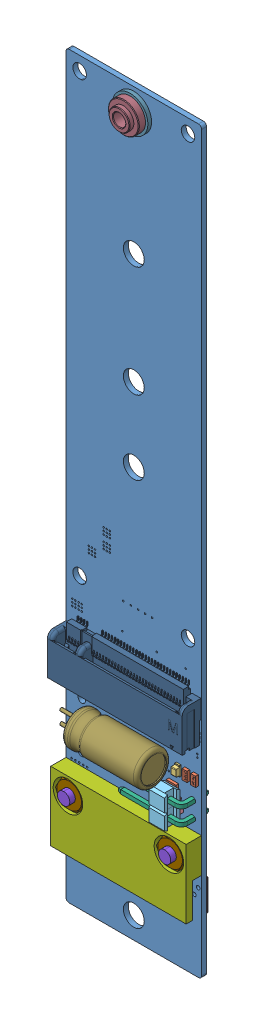
SolidWorks assembly R44SF ..22, configuration 默认. Lengths in mm.
Overall size (46.94 221.57 8.14).
41 component instances, 17 part files, 0 mates.
Components (placement in the parent):
- R44SF ..22.step-1: R44SF ..22.step [默认] at origin size (22.08 211.37 8.14)
  - Board.step-1: Board.step [默认] at origin size (22.06 211.37 0.8)
    - Open CASCADE STEP translator 6.8 12.1.1.step-1: Open CASCADE STEP translator 6.8 12.1.1.step [默认] at (0 0 -0.8) size (22.06 211.37 0.8)
  - R3.step-1: R3.step [默认] at origin size (1.6 0.8 0.45)
    - ________R0603.step-1: ________R0603.step [默认] at (119.5501 177.9636 0) x (1 0 0) z (0 0 1) size (1.6 0.8 0.45)
      - ________R0603-0.step-1: ________R0603-0.step [默认] at origin size (1.6 0.8 0.45)
  - D1.step-1: D1.step [默认] at origin size (0.8 1.6 1.1)
    - LED_AP1608.step-1: LED_AP1608.step [默认] at (120.3536 180.4092 0) x (0 1 0) z (1 0 0) size (1.6 1.1 0.8)
  - R2.step-1: R2.step [默认] at origin size (0.8 1.6 0.45)
    - ________R0603.step-1: ________R0603.step [默认] at (121.7526 180.421 0) x (0 -1 0) z (0 0 1) size (1.6 0.8 0.45)
      - ________R0603-0.step-1: ________R0603-0.step [默认] at origin size (1.6 0.8 0.45)
  - R1.step-1: R1.step [默认] at origin size (0.8 1.6 0.45)
    - ________R0603.step-1: ________R0603.step [默认] at (123.1496 180.421 0) x (0 -1 0) z (0 0 1) size (1.6 0.8 0.45)
      - ________R0603-0.step-1: ________R0603-0.step [默认] at origin size (1.6 0.8 0.45)
  - Q1.step-1: Q1.step [默认] at origin size (3 2.55 1)
    - SOT-23.step-1: SOT-23.step [默认] at (113.165 176.0289 0) x (-1 0 0) z (0 0 1) size (3 2.55 1)
  - Free-Models.step-1: Free-Models.step [默认] at origin size (22.08 200.73 8.14)
    - bg075-02x-1-0600-0300-0150-x-x_revd.step-1: bg075-02x-1-0600-0300-0150-x-x_revd.step [默认] at (120.1725 176.0952 0.5) x (0 -1 0) z (0 0 -1) size (5.08 10.36 5.5)
      - BG075-Insulator.step-1: BG075-Insulator.step [默认] at (0.3712 -0.9743 -0.1079) size (2.54 2.54 2.5)
      - BG075-Insulator.step-2: BG075-Insulator.step [默认] at (-2.1688 -0.9743 -0.1079) size (2.54 2.54 2.5)
      - BG075-1-0600-0300-0150-pin.step-1: BG075-1-0600-0300-0150-pin.step [默认] at (1.0892 -2.7943 -1.0379) size (0.64 10.36 4.57)
      - BG075-1-0600-0300-0150-pin.step-2: BG075-1-0600-0300-0150-pin.step [默认] at (-1.4508 -2.7943 -1.0379) size (0.64 10.36 4.57)
    - RP44S-PAD.step-1: RP44S-PAD.step [默认] at (102.0666 172.9244 2.5) x (-1 0 0) z (0 -1 0) size (22 2.5 11.2)
    - G0033_RGB9411503.step-1: G0033_RGB9411503.step [默认] at (121.2666 170.1244 -1.8) x (-1 0 0) z (0 1 0) size (3.3 5 3.3)
    - Hexagon_nut_ISO_4032_(DIN_934)_-_M2_RGB9411503.step-1: Hexagon_nut_ISO_4032_(DIN_934)_-_M2_RGB9411503.step [默认] at (121.2666 170.1244 1.5) x (-1 0 0) z (0 1 0) size (4.63 1.61 4.63)
    - Hexagon_nut_ISO_4032_(DIN_934)_-_M2_RGB9411503.step-2: Hexagon_nut_ISO_4032_(DIN_934)_-_M2_RGB9411503.step [默认] at (104.8666 170.1274 1.5) x (-1 0 0) z (0 1 0) size (4.63 1.61 4.63)
    - G0033_RGB9411503.step-2: G0033_RGB9411503.step [默认] at (104.8666 170.1274 -1.8) x (-1 0 0) z (0 1 0) size (3.3 5 3.3)
    - c-1-2199119-3-a1-3d_RGB4404530.step-1: c-1-2199119-3-a1-3d_RGB4404530.step [默认] at (113.0625 193.4584 1.7) x (-1 0 0) z (0 1 0) size (21.9 3.7 8.7)
    - Tape_22x5_RGB0.step-1: Tape_22x5_RGB0.step [默认] at (102.119 161.6272 -1) x (1 0 0) z (0 0 1) size (22 5 0.1)
    - CAP_RAD_D5x11_POL_BK.step-1: CAP_RAD_D5x11_POL_BK.step [默认] at (106.7892 181.2957 3) x (0 -1 0) z (1 0 0) size (5.5 5.5 15.01)
    - M2_nuc_RGB3326705.step-1: M2_nuc_RGB3326705.step [默认] at (113.0667 269.231 -1.1) x (1 0 0) z (0 -1 0) size (5 3.5 5)
    - G0042.step-1: G0042.step [默认] at (113.0667 269.231 0) x (1 0 0) z (0 -1 0) size (5.76 0.6 5.76)
    - G0042.step-2: G0042.step [默认] at (113.0667 269.231 -1.4) x (1 0 0) z (0 -1 0) size (5.76 0.6 5.76)
    - G0030_RGB12967653.step-1: G0030_RGB12967653.step [默认] at (113.0666 269.231 -1.9) x (1 0 0) z (0 -1 0) size (4.1 2.43 4.1)
    - G0033_RGB9411503.step-3: G0033_RGB9411503.step [默认] at (121.272 74.174 -1.8) x (1 0 0) z (0 -1 0) size (3.3 5 3.3) (hidden)
    - Hexagon_nut_ISO_4032_(DIN_934)_-_M2_RGB9411503.step-3: Hexagon_nut_ISO_4032_(DIN_934)_-_M2_RGB9411503.step [默认] at (121.272 74.174 1.5) x (1 0 0) z (0 -1 0) size (4.63 1.61 4.63) (hidden)
    - Hexagon_nut_ISO_4032_(DIN_934)_-_M2_RGB9411503.step-4: Hexagon_nut_ISO_4032_(DIN_934)_-_M2_RGB9411503.step [默认] at (104.872 74.177 1.5) x (1 0 0) z (0 -1 0) size (4.63 1.61 4.63) (hidden)
    - G0033_RGB9411503.step-4: G0033_RGB9411503.step [默认] at (104.872 74.177 -1.8) x (1 0 0) z (0 -1 0) size (3.3 5 3.3) (hidden)
    - RP44S-PAD.step-2: RP44S-PAD.step [默认] at (124.0685 71.3783 2.5) x (1 0 0) z (0 1 0) size (22 2.5 11.2) (hidden)
    - cable13-83.step-1: cable13-83.step [默认] at (102.6059 80.1574 1.4) x (-1 0 0) z (0 1 0) size (8.76 2.1 87.74) (hidden)
    - cable20-83.step-1: cable20-83.step [默认] at (111.4616 80.1574 1.4) x (1 0 0) z (0 -1 0) size (13.2 2.1 87.74) (hidden)
